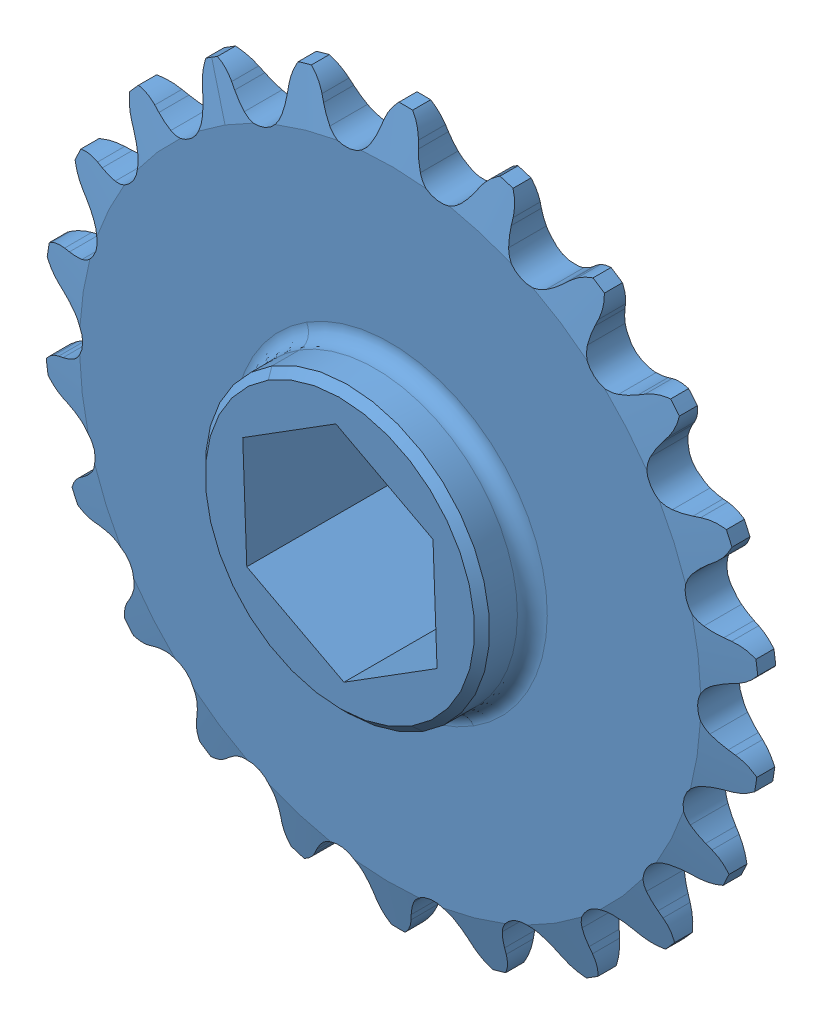
SolidWorks assembly WCP - GreyT Elevator (Cascade, 2 Stage) (1).step, configuration Default. Lengths in mm.
Overall size (65.87 65.96 9.52).
407 component instances, 66 part files, 0 mates.
Components (placement in the parent):
- WCP-0323 - Elevator Clamping Block.step-1: WCP-0323 - Elevator Clamping Block.step [Default] at (152.3365 1149.35 -25.4) x (0 0 1) z (-1 0 0) size (29.22 25.41 49.35) (hidden)
  - WCP-0323-001 Rev2.step-1: WCP-0323-001 Rev2.step [Default] at origin size (20.38 25.41 40.49)
  - WCP-0498 Rev1.step-1: WCP-0498 Rev1.step [Default] at (2.254 0 6.7) x (0 0.307359 0.951594) z (-1 0 0) size (12 12 4)
  - WCP-0212_0_250_radial_bearing.step-1: WCP-0212_0_250_radial_bearing.step [Default] at (-9.525 0 15.4781) size (19.05 19.05 7.14)
  - WCP-0473 Rev1.step-1: WCP-0473 Rev1.step [Default] at (-9.525 0 10.4394) x (-0.082744 -0.996571 0) z (-0.996571 0.082744 0) size (9.53 20.65 9.53)
  - #8-32 x .25L BHCS.step-1: #8-32 x .25L BHCS.step [Default] at (6.7178 0 6.7) x (0 -0.337236 -0.94142) z (1 0 0) size (10.28 8 12.02)
- WCP-0323 - Elevator Clamping Block-1.step-1: WCP-0323 - Elevator Clamping Block-1.step [Default] at (152.3365 1149.35 25.4) x (0 0 -1) z (-1 0 0) size (29.22 25.41 49.35) (hidden)
  - WCP-0323-001 Rev2.step-1: WCP-0323-001 Rev2.step [Default] at origin size (20.38 25.41 40.49)
  - WCP-0498 Rev1.step-1: WCP-0498 Rev1.step [Default] at (2.254 0 6.7) x (0 0.307359 0.951594) z (-1 0 0) size (12 12 4)
  - WCP-0212_0_250_radial_bearing.step-1: WCP-0212_0_250_radial_bearing.step [Default] at (-9.525 0 15.4781) size (19.05 19.05 7.14)
  - WCP-0473 Rev1.step-1: WCP-0473 Rev1.step [Default] at (-9.525 0 10.4394) x (-0.082744 -0.996571 0) z (-0.996571 0.082744 0) size (9.53 20.65 9.53)
  - #8-32 x .25L BHCS.step-1: #8-32 x .25L BHCS.step [Default] at (6.7178 0 6.7) x (0 -0.337236 -0.94142) z (1 0 0) size (10.28 8 12.02)
- WCP-0323 - Elevator Clamping Block-2.step-1: WCP-0323 - Elevator Clamping Block-2.step [Default] at (139.7635 57.15 25.4) x (0 0 -1) z (1 0 0) size (29.22 25.41 49.35) (hidden)
  - WCP-0323-001 Rev2.step-1: WCP-0323-001 Rev2.step [Default] at origin size (20.38 25.41 40.49)
  - WCP-0498 Rev1.step-1: WCP-0498 Rev1.step [Default] at (2.254 0 6.7) x (0 0.307359 0.951594) z (-1 0 0) size (12 12 4)
  - WCP-0212_0_250_radial_bearing.step-1: WCP-0212_0_250_radial_bearing.step [Default] at (-9.525 0 15.4781) size (19.05 19.05 7.14)
  - WCP-0473 Rev1.step-1: WCP-0473 Rev1.step [Default] at (-9.525 0 10.4394) x (-0.082744 -0.996571 0) z (-0.996571 0.082744 0) size (9.53 20.65 9.53)
  - #8-32 x .25L BHCS.step-1: #8-32 x .25L BHCS.step [Default] at (6.7178 0 6.7) x (0 -0.337236 -0.94142) z (1 0 0) size (10.28 8 12.02)
- WCP-0323 - Elevator Clamping Block-3.step-1: WCP-0323 - Elevator Clamping Block-3.step [Default] at (139.7635 57.15 -25.4) x (0 0 1) z (1 0 0) size (29.22 25.41 49.35) (hidden)
  - WCP-0323-001 Rev2.step-1: WCP-0323-001 Rev2.step [Default] at origin size (20.38 25.41 40.49)
  - WCP-0498 Rev1.step-1: WCP-0498 Rev1.step [Default] at (2.254 0 6.7) x (0 0.307359 0.951594) z (-1 0 0) size (12 12 4)
  - WCP-0212_0_250_radial_bearing.step-1: WCP-0212_0_250_radial_bearing.step [Default] at (-9.525 0 15.4781) size (19.05 19.05 7.14)
  - WCP-0473 Rev1.step-1: WCP-0473 Rev1.step [Default] at (-9.525 0 10.4394) x (-0.082744 -0.996571 0) z (-0.996571 0.082744 0) size (9.53 20.65 9.53)
  - #8-32 x .25L BHCS.step-1: #8-32 x .25L BHCS.step [Default] at (6.7178 0 6.7) x (0 -0.337236 -0.94142) z (1 0 0) size (10.28 8 12.02)
- WCP-0323 - Elevator Clamping Block-4.step-1: WCP-0323 - Elevator Clamping Block-4.step [Default] at (101.6635 82.55 25.4) x (0 0 -1) z (1 0 0) size (29.22 25.41 49.35) (hidden)
  - WCP-0323-001 Rev2.step-1: WCP-0323-001 Rev2.step [Default] at origin size (20.38 25.41 40.49)
  - WCP-0498 Rev1.step-1: WCP-0498 Rev1.step [Default] at (2.254 0 6.7) x (0 0.307359 0.951594) z (-1 0 0) size (12 12 4)
  - WCP-0212_0_250_radial_bearing.step-1: WCP-0212_0_250_radial_bearing.step [Default] at (-9.525 0 15.4781) size (19.05 19.05 7.14)
  - WCP-0473 Rev1.step-1: WCP-0473 Rev1.step [Default] at (-9.525 0 10.4394) x (-0.082744 -0.996571 0) z (-0.996571 0.082744 0) size (9.53 20.65 9.53)
  - #8-32 x .25L BHCS.step-1: #8-32 x .25L BHCS.step [Default] at (6.7178 0 6.7) x (0 -0.337236 -0.94142) z (1 0 0) size (10.28 8 12.02)
- WCP-0323 - Elevator Clamping Block-5.step-1: WCP-0323 - Elevator Clamping Block-5.step [Default] at (101.6635 82.55 -25.4) x (0 0 1) z (1 0 0) size (29.22 25.41 49.35) (hidden)
  - WCP-0323-001 Rev2.step-1: WCP-0323-001 Rev2.step [Default] at origin size (20.38 25.41 40.49)
  - WCP-0498 Rev1.step-1: WCP-0498 Rev1.step [Default] at (2.254 0 6.7) x (0 0.307359 0.951594) z (-1 0 0) size (12 12 4)
  - WCP-0212_0_250_radial_bearing.step-1: WCP-0212_0_250_radial_bearing.step [Default] at (-9.525 0 15.4781) size (19.05 19.05 7.14)
  - WCP-0473 Rev1.step-1: WCP-0473 Rev1.step [Default] at (-9.525 0 10.4394) x (-0.082744 -0.996571 0) z (-0.996571 0.082744 0) size (9.53 20.65 9.53)
  - #8-32 x .25L BHCS.step-1: #8-32 x .25L BHCS.step [Default] at (6.7178 0 6.7) x (0 -0.337236 -0.94142) z (1 0 0) size (10.28 8 12.02)
- WCP-0323 - Elevator Clamping Block-6.step-1: WCP-0323 - Elevator Clamping Block-6.step [Default] at (101.6635 222.25 25.4) x (0 0 -1) z (1 0 0) size (29.22 25.41 49.35) (hidden)
  - WCP-0323-001 Rev2.step-1: WCP-0323-001 Rev2.step [Default] at origin size (20.38 25.41 40.49)
  - WCP-0498 Rev1.step-1: WCP-0498 Rev1.step [Default] at (2.254 0 6.7) x (0 0.307359 0.951594) z (-1 0 0) size (12 12 4)
  - WCP-0212_0_250_radial_bearing.step-1: WCP-0212_0_250_radial_bearing.step [Default] at (-9.525 0 15.4781) size (19.05 19.05 7.14)
  - WCP-0473 Rev1.step-1: WCP-0473 Rev1.step [Default] at (-9.525 0 10.4394) x (-0.082744 -0.996571 0) z (-0.996571 0.082744 0) size (9.53 20.65 9.53)
  - #8-32 x .25L BHCS.step-1: #8-32 x .25L BHCS.step [Default] at (6.7178 0 6.7) x (0 -0.337236 -0.94142) z (1 0 0) size (10.28 8 12.02)
- WCP-0323 - Elevator Clamping Block-7.step-1: WCP-0323 - Elevator Clamping Block-7.step [Default] at (101.6635 222.25 -25.4) x (0 0 1) z (1 0 0) size (29.22 25.41 49.35) (hidden)
  - WCP-0323-001 Rev2.step-1: WCP-0323-001 Rev2.step [Default] at origin size (20.38 25.41 40.49)
  - WCP-0498 Rev1.step-1: WCP-0498 Rev1.step [Default] at (2.254 0 6.7) x (0 0.307359 0.951594) z (-1 0 0) size (12 12 4)
  - WCP-0212_0_250_radial_bearing.step-1: WCP-0212_0_250_radial_bearing.step [Default] at (-9.525 0 15.4781) size (19.05 19.05 7.14)
  - WCP-0473 Rev1.step-1: WCP-0473 Rev1.step [Default] at (-9.525 0 10.4394) x (-0.082744 -0.996571 0) z (-0.996571 0.082744 0) size (9.53 20.65 9.53)
  - #8-32 x .25L BHCS.step-1: #8-32 x .25L BHCS.step [Default] at (6.7178 0 6.7) x (0 -0.337236 -0.94142) z (1 0 0) size (10.28 8 12.02)
- WCP-0248 Rev1 - #35 Chain Turnbuckle.step-1: WCP-0248 Rev1 - #35 Chain Turnbuckle.step [Default] at (88.9 1124.7437 -66.675) x (0 -1 0) z (0 0 1) size (55.56 15.05 15.04) (hidden)
  - WCP-0247-001 Rev1.step-1: WCP-0247-001 Rev1.step [Default] at origin size (30.16 9.53 11)
  - NFS-0040_#10-32_jam_nut_left_hand_99961A520.step-1: NFS-0040_#10-32_jam_nut_left_hand_99961A520.step [Default] at (-16.6687 0 0) x (0 0.5 -0.866025) z (0 0.866025 0.5) size (11.01 3.2 11.02)
  - NFS-0037_#10-32_jam_nut_90480A195.step-1: NFS-0037_#10-32_jam_nut_90480A195.step [Default] at (16.6687 0 0) x (0 0.5 0.866025) z (0 -0.866025 0.5) size (11.01 3.2 11.02)
  - WCP-0248-001 Rev1.step-1: WCP-0248-001 Rev1.step [Default] at (23.8125 0 0) x (0 0 1) z (0 1 0) size (9 25.4 9)
  - WCP-0248-002 Rev1.step-1: WCP-0248-002 Rev1.step [Default] at (-23.8125 0 0) x (0 0 -1) z (0 1 0) size (9 25.4 9)
- WCP-0247 Rev1 - #25 Chain Turnbuckle.step-1: WCP-0247 Rev1 - #25 Chain Turnbuckle.step [Default] at (-47.6339 1117.6 -50.8) x (0 1 0) z (-1 0 0) size (50.8 15.05 15.04) (hidden)
  - WCP-0247-001 Rev1.step-1: WCP-0247-001 Rev1.step [Default] at origin size (30.16 9.53 11)
  - NFS-0040_#10-32_jam_nut_left_hand_99961A520.step-1: NFS-0040_#10-32_jam_nut_left_hand_99961A520.step [Default] at (-16.6687 0 0) x (0 0.5 -0.866025) z (0 0.866025 0.5) size (11.01 3.2 11.02)
  - NFS-0037_#10-32_jam_nut_90480A195.step-1: NFS-0037_#10-32_jam_nut_90480A195.step [Default] at (16.6687 0 0) x (0 0.5 0.866025) z (0 -0.866025 0.5) size (11.01 3.2 11.02)
  - WCP-0247-002 Rev2.step-1: WCP-0247-002 Rev2.step [Default] at (22.225 0 0) x (0 0 1) z (0 1 0) size (9 23.02 5.21)
  - WCP-0247-003 Rev2.step-1: WCP-0247-003 Rev2.step [Default] at (-22.225 0 0) x (0 0 -1) z (0 1 0) size (9 23.02 5.21)
- WCP-0323 - Elevator Clamping Block-8.step-1: WCP-0323 - Elevator Clamping Block-8.step [Default] at (-152.3365 1149.35 25.4) x (0 0 -1) z (1 0 0) size (29.22 25.41 49.35) (hidden)
  - WCP-0323-001 Rev2.step-1: WCP-0323-001 Rev2.step [Default] at origin size (20.38 25.41 40.49)
  - WCP-0498 Rev1.step-1: WCP-0498 Rev1.step [Default] at (2.254 0 6.7) x (0 0.307359 0.951594) z (-1 0 0) size (12 12 4)
  - WCP-0212_0_250_radial_bearing.step-1: WCP-0212_0_250_radial_bearing.step [Default] at (-9.525 0 15.4781) size (19.05 19.05 7.14)
  - WCP-0473 Rev1.step-1: WCP-0473 Rev1.step [Default] at (-9.525 0 10.4394) x (-0.082744 -0.996571 0) z (-0.996571 0.082744 0) size (9.53 20.65 9.53)
  - #8-32 x .25L BHCS.step-1: #8-32 x .25L BHCS.step [Default] at (6.7178 0 6.7) x (0 -0.337236 -0.94142) z (1 0 0) size (10.28 8 12.02)
- WCP-0323 - Elevator Clamping Block-9.step-1: WCP-0323 - Elevator Clamping Block-9.step [Default] at (-152.3365 1149.35 -25.4) x (0 0 1) z (1 0 0) size (29.22 25.41 49.35) (hidden)
  - WCP-0323-001 Rev2.step-1: WCP-0323-001 Rev2.step [Default] at origin size (20.38 25.41 40.49)
  - WCP-0498 Rev1.step-1: WCP-0498 Rev1.step [Default] at (2.254 0 6.7) x (0 0.307359 0.951594) z (-1 0 0) size (12 12 4)
  - WCP-0212_0_250_radial_bearing.step-1: WCP-0212_0_250_radial_bearing.step [Default] at (-9.525 0 15.4781) size (19.05 19.05 7.14)
  - WCP-0473 Rev1.step-1: WCP-0473 Rev1.step [Default] at (-9.525 0 10.4394) x (-0.082744 -0.996571 0) z (-0.996571 0.082744 0) size (9.53 20.65 9.53)
  - #8-32 x .25L BHCS.step-1: #8-32 x .25L BHCS.step [Default] at (6.7178 0 6.7) x (0 -0.337236 -0.94142) z (1 0 0) size (10.28 8 12.02)
- WCP-0583 Rev1 - Cascade Pulley Block.step-1: WCP-0583 Rev1 - Cascade Pulley Block.step [Default] at (88.9 25.4 -25.4) x (1 0 0) z (0 1 0) size (47.02 52.05 52.05) (hidden)
  - WCP-0096 Rev6.step-1: WCP-0096 Rev6.step [Default] at (0 25.4 6.35) size (12.65 52.05 52.05)
    - WCP-0096-001 Rev6.step-1: WCP-0096-001 Rev6.step [Default] at origin size (7.57 38.1 38.1)
    - WCP-0096-001 Rev6.step-2: WCP-0096-001 Rev6.step [Default] x (-1 0 0) z (0 0.866025 -0.5) size (7.57 38.1 38.1)
    - WCP-0356 Rev1.step-1: WCP-0356 Rev1.step [Default] at (0.4817 -4.7625 -8.2489) x (0 -0.126969 0.991907) z (0 -0.991907 -0.126969) size (4.06 11.05 4.06)
    - WCP-0356 Rev1.step-2: WCP-0356 Rev1.step [Default] at (0.4817 9.525 0) x (0 0.866766 0.498715) z (0 -0.498715 0.866766) size (4.06 11.05 4.06)
    - WCP-0356 Rev1.step-3: WCP-0356 Rev1.step [Default] at (0.4817 -4.7625 8.2489) x (0 -0.994015 -0.109248) z (0 0.109248 -0.994015) size (4.06 11.05 4.06)
    - WCP-0356 Rev1.step-4: WCP-0356 Rev1.step [Default] at (-0.4817 4.7625 -8.2489) x (0 -0.997555 0.069879) z (0 0.069879 0.997555) size (4.06 11.05 4.06)
    - WCP-0356 Rev1.step-5: WCP-0356 Rev1.step [Default] at (-0.4817 4.7625 8.2489) x (0 -0.7202 -0.693767) z (0 -0.693767 0.7202) size (4.06 11.05 4.06)
    - WCP-0356 Rev1.step-6: WCP-0356 Rev1.step [Default] at (-0.4817 -9.525 0) x (0 -0.997555 0.069879) z (0 0.069879 0.997555) size (4.06 11.05 4.06)
  - WCP-0583-001 Rev1.step-1: WCP-0583-001 Rev1.step [Default] at origin size (34.92 31.75 25.4)
  - WCP-0567 Rev1.step-1: WCP-0567 Rev1.step [Default] at (-6.3246 25.4 6.35) x (0 0 1) z (-1 0 0) size (15.88 15.88 7.94)
  - WCP-0567 Rev1.step-2: WCP-0567 Rev1.step [Default] at (6.3246 25.4 6.35) x (0 0 1) z (1 0 0) size (15.88 15.88 7.94)
  - WCP-0203 Rev1.step-1: WCP-0203 Rev1.step [Default] at (0 25.4 6.35) size (15.88 9.5 9.5)
  - 10-32 BHCS - No Thread_WCP-0258 - 1.750.step-1: 10-32 BHCS - No Thread_WCP-0258 - 1.750.step [Default] at (-17.4625 25.4 6.35) x (0 -0.816967 0.576685) z (0 -0.576685 -0.816967) size (9.17 47.02 9.17)
  - WCP-0326 Rev1.step-1: WCP-0326 Rev1.step [Default] at (19.8374 25.4 6.35) x (0 0.003214 -0.999995) z (0 -0.999995 -0.003214) size (11.02 4.76 11)
- WCP-0583 Rev1 - Cascade Pulley Block-1.step-1: WCP-0583 Rev1 - Cascade Pulley Block-1.step [Default] at (88.9 1219.2 -25.4) x (1 0 0) z (0 1 0) size (47.02 52.05 52.05) (hidden)
  - WCP-0096 Rev6-1.step-1: WCP-0096 Rev6-1.step [Default] at (0 25.4 6.35) size (12.65 52.05 52.05)
    - WCP-0096-001 Rev6.step-1: WCP-0096-001 Rev6.step [Default] at origin size (7.57 38.1 38.1)
    - WCP-0096-001 Rev6.step-2: WCP-0096-001 Rev6.step [Default] x (-1 0 0) z (0 0.866025 -0.5) size (7.57 38.1 38.1)
    - WCP-0356 Rev1.step-1: WCP-0356 Rev1.step [Default] at (0.4817 -4.7625 -8.2489) x (0 -0.126969 0.991907) z (0 -0.991907 -0.126969) size (4.06 11.05 4.06)
    - WCP-0356 Rev1.step-2: WCP-0356 Rev1.step [Default] at (0.4817 9.525 0) x (0 0.866766 0.498715) z (0 -0.498715 0.866766) size (4.06 11.05 4.06)
    - WCP-0356 Rev1.step-3: WCP-0356 Rev1.step [Default] at (0.4817 -4.7625 8.2489) x (0 -0.994015 -0.109248) z (0 0.109248 -0.994015) size (4.06 11.05 4.06)
    - WCP-0356 Rev1.step-4: WCP-0356 Rev1.step [Default] at (-0.4817 4.7625 -8.2489) x (0 -0.997555 0.069879) z (0 0.069879 0.997555) size (4.06 11.05 4.06)
    - WCP-0356 Rev1.step-5: WCP-0356 Rev1.step [Default] at (-0.4817 4.7625 8.2489) x (0 -0.7202 -0.693767) z (0 -0.693767 0.7202) size (4.06 11.05 4.06)
    - WCP-0356 Rev1.step-6: WCP-0356 Rev1.step [Default] at (-0.4817 -9.525 0) x (0 -0.997555 0.069879) z (0 0.069879 0.997555) size (4.06 11.05 4.06)
  - WCP-0583-001 Rev1.step-1: WCP-0583-001 Rev1.step [Default] at origin size (34.92 31.75 25.4)
  - WCP-0567 Rev1.step-1: WCP-0567 Rev1.step [Default] at (-6.3246 25.4 6.35) x (0 0 1) z (-1 0 0) size (15.88 15.88 7.94)
  - WCP-0567 Rev1.step-2: WCP-0567 Rev1.step [Default] at (6.3246 25.4 6.35) x (0 0 1) z (1 0 0) size (15.88 15.88 7.94)
  - WCP-0203 Rev1.step-1: WCP-0203 Rev1.step [Default] at (0 25.4 6.35) size (15.88 9.5 9.5)
  - 10-32 BHCS - No Thread_WCP-0258 - 1.750.step-1: 10-32 BHCS - No Thread_WCP-0258 - 1.750.step [Default] at (-17.4625 25.4 6.35) x (0 -0.816967 0.576685) z (0 -0.576685 -0.816967) size (9.17 47.02 9.17)
  - WCP-0326 Rev1.step-1: WCP-0326 Rev1.step [Default] at (19.8374 25.4 6.35) x (0 0.003214 -0.999995) z (0 -0.999995 -0.003214) size (11.02 4.76 11)
- WCP-0583 Rev1 - Cascade Pulley Block_Mirrored.step-1: WCP-0583 Rev1 - Cascade Pulley Block_Mirrored.step [Default] at (-88.9 1219.2 -25.4) x (1 0 0) z (0 1 0) size (47.02 52.05 52.05) (hidden)
  - WCP-0096 Rev6-2.step-1: WCP-0096 Rev6-2.step [Default] at (0 25.4 6.35) size (12.65 52.05 52.05)
    - WCP-0096-001 Rev6.step-1: WCP-0096-001 Rev6.step [Default] at origin size (7.57 38.1 38.1)
    - WCP-0096-001 Rev6.step-2: WCP-0096-001 Rev6.step [Default] x (-1 0 0) z (0 0.866025 -0.5) size (7.57 38.1 38.1)
    - WCP-0356 Rev1.step-1: WCP-0356 Rev1.step [Default] at (0.4817 -4.7625 -8.2489) x (0 -0.126969 0.991907) z (0 -0.991907 -0.126969) size (4.06 11.05 4.06)
    - WCP-0356 Rev1.step-2: WCP-0356 Rev1.step [Default] at (0.4817 9.525 0) x (0 0.866766 0.498715) z (0 -0.498715 0.866766) size (4.06 11.05 4.06)
    - WCP-0356 Rev1.step-3: WCP-0356 Rev1.step [Default] at (0.4817 -4.7625 8.2489) x (0 -0.994015 -0.109248) z (0 0.109248 -0.994015) size (4.06 11.05 4.06)
    - WCP-0356 Rev1.step-4: WCP-0356 Rev1.step [Default] at (-0.4817 4.7625 -8.2489) x (0 -0.997555 0.069879) z (0 0.069879 0.997555) size (4.06 11.05 4.06)
    - WCP-0356 Rev1.step-5: WCP-0356 Rev1.step [Default] at (-0.4817 4.7625 8.2489) x (0 -0.7202 -0.693767) z (0 -0.693767 0.7202) size (4.06 11.05 4.06)
    - WCP-0356 Rev1.step-6: WCP-0356 Rev1.step [Default] at (-0.4817 -9.525 0) x (0 -0.997555 0.069879) z (0 0.069879 0.997555) size (4.06 11.05 4.06)
  - WCP-0583-001 Rev1.step-1: WCP-0583-001 Rev1.step [Default] at origin size (34.92 31.75 25.4)
  - WCP-0567 Rev1.step-1: WCP-0567 Rev1.step [Default] at (-6.3246 25.4 6.35) x (0 0 1) z (-1 0 0) size (15.88 15.88 7.94)
  - WCP-0567 Rev1.step-2: WCP-0567 Rev1.step [Default] at (6.3246 25.4 6.35) x (0 0 1) z (1 0 0) size (15.88 15.88 7.94)
  - WCP-0203 Rev1.step-1: WCP-0203 Rev1.step [Default] at (0 25.4 6.35) size (15.88 9.5 9.5)
  - 10-32 BHCS - No Thread_WCP-0258 - 1.750.step-1: 10-32 BHCS - No Thread_WCP-0258 - 1.750.step [Default] at (17.4625 25.4 6.35) x (0 0.844944 -0.534854) z (0 -0.534854 -0.844944) size (9.17 47.02 9.17)
  - WCP-0326 Rev1.step-1: WCP-0326 Rev1.step [Default] at (-19.8374 25.4 6.35) x (0 -0.925447 -0.378877) z (0 0.378877 -0.925447) size (11.02 4.76 11)
- WCP-0583 Rev1 - Cascade Pulley Block_Mirrored-1.step-1: WCP-0583 Rev1 - Cascade Pulley Block_Mirrored-1.step [Default] at (-88.9 25.4 -25.4) x (1 0 0) z (0 1 0) size (47.02 52.05 52.05) (hidden)
  - WCP-0096 Rev6-3.step-1: WCP-0096 Rev6-3.step [Default] at (0 25.4 6.35) size (12.65 52.05 52.05)
    - WCP-0096-001 Rev6.step-1: WCP-0096-001 Rev6.step [Default] at origin size (7.57 38.1 38.1)
    - WCP-0096-001 Rev6.step-2: WCP-0096-001 Rev6.step [Default] x (-1 0 0) z (0 0.866025 -0.5) size (7.57 38.1 38.1)
    - WCP-0356 Rev1.step-1: WCP-0356 Rev1.step [Default] at (0.4817 -4.7625 -8.2489) x (0 -0.126969 0.991907) z (0 -0.991907 -0.126969) size (4.06 11.05 4.06)
    - WCP-0356 Rev1.step-2: WCP-0356 Rev1.step [Default] at (0.4817 9.525 0) x (0 0.866766 0.498715) z (0 -0.498715 0.866766) size (4.06 11.05 4.06)
    - WCP-0356 Rev1.step-3: WCP-0356 Rev1.step [Default] at (0.4817 -4.7625 8.2489) x (0 -0.994015 -0.109248) z (0 0.109248 -0.994015) size (4.06 11.05 4.06)
    - WCP-0356 Rev1.step-4: WCP-0356 Rev1.step [Default] at (-0.4817 4.7625 -8.2489) x (0 -0.997555 0.069879) z (0 0.069879 0.997555) size (4.06 11.05 4.06)
    - WCP-0356 Rev1.step-5: WCP-0356 Rev1.step [Default] at (-0.4817 4.7625 8.2489) x (0 -0.7202 -0.693767) z (0 -0.693767 0.7202) size (4.06 11.05 4.06)
    - WCP-0356 Rev1.step-6: WCP-0356 Rev1.step [Default] at (-0.4817 -9.525 0) x (0 -0.997555 0.069879) z (0 0.069879 0.997555) size (4.06 11.05 4.06)
  - WCP-0583-001 Rev1.step-1: WCP-0583-001 Rev1.step [Default] at origin size (34.92 31.75 25.4)
  - WCP-0567 Rev1.step-1: WCP-0567 Rev1.step [Default] at (-6.3246 25.4 6.35) x (0 0 1) z (-1 0 0) size (15.88 15.88 7.94)
  - WCP-0567 Rev1.step-2: WCP-0567 Rev1.step [Default] at (6.3246 25.4 6.35) x (0 0 1) z (1 0 0) size (15.88 15.88 7.94)
  - WCP-0203 Rev1.step-1: WCP-0203 Rev1.step [Default] at (0 25.4 6.35) size (15.88 9.5 9.5)
  - 10-32 BHCS - No Thread_WCP-0258 - 1.750.step-1: 10-32 BHCS - No Thread_WCP-0258 - 1.750.step [Default] at (17.4625 25.4 6.35) x (0 0.844944 -0.534854) z (0 -0.534854 -0.844944) size (9.17 47.02 9.17)
  - WCP-0326 Rev1.step-1: WCP-0326 Rev1.step [Default] at (-19.8374 25.4 6.35) x (0 -0.925447 -0.378877) z (0 0.378877 -0.925447) size (11.02 4.76 11)
- WCP-0323 - Elevator Clamping Block-10.step-1: WCP-0323 - Elevator Clamping Block-10.step [Default] at (-139.7635 57.15 -25.4) x (0 0 1) z (-1 0 0) size (29.22 25.41 49.35) (hidden)
  - WCP-0323-001 Rev2.step-1: WCP-0323-001 Rev2.step [Default] at origin size (20.38 25.41 40.49)
  - WCP-0498 Rev1.step-1: WCP-0498 Rev1.step [Default] at (2.254 0 6.7) x (0 0.307359 0.951594) z (-1 0 0) size (12 12 4)
  - WCP-0212_0_250_radial_bearing.step-1: WCP-0212_0_250_radial_bearing.step [Default] at (-9.525 0 15.4781) size (19.05 19.05 7.14)
  - WCP-0473 Rev1.step-1: WCP-0473 Rev1.step [Default] at (-9.525 0 10.4394) x (-0.082744 -0.996571 0) z (-0.996571 0.082744 0) size (9.53 20.65 9.53)
  - #8-32 x .25L BHCS.step-1: #8-32 x .25L BHCS.step [Default] at (6.7178 0 6.7) x (0 -0.337236 -0.94142) z (1 0 0) size (10.28 8 12.02)
- WCP-0557 Rev1 - WCP Single Stage Gearbox_0.5_ Hex.step-1: WCP-0557 Rev1 - WCP Single Stage Gearbox_0.5_ Hex.step [Default] at (-25.4 0 66.675) x (-1 0 0) z (0 0 -1) size (173.55 82.41 254.05) (hidden)
  - WCP-0557-001 Rev1.step-1: WCP-0557-001 Rev1.step [Default] at origin size (151.92 76.2 6.35)
  - WCP-0557-002 Rev1.step-1: WCP-0557-002 Rev1.step [Default] at (0 0 34.925) size (76.2 76.2 6.35)
  - 217-6515_Falcon_500_Default_As Machined_.step-1: 217-6515_Falcon_500_Default_As Machined_.step [Default] at (45.7962 0 -29.375) x (0.866025 0.5 0) z (0 0 1) size (60 60 115.81)
  - 217-6515_Falcon_500_Default_As Machined_.step-2: 217-6515_Falcon_500_Default_As Machined_.step [Default] at (-45.7962 0 -29.375) x (0.866025 0.5 0) z (0 0 1) size (60 60 115.81)
  - 217-6919_Falcon_12T.step-1: 217-6919_Falcon_12T.step [Default] at (45.7962 0 12.5775) x (0.990666 -0.136309 0) z (0 0 1) size (17.78 17.78 19.05)
  - 217-6919_Falcon_12T.step-2: 217-6919_Falcon_12T.step [Default] at (-45.7962 0 12.5775) x (0.990666 -0.136309 0) z (0 0 1) size (17.78 17.78 19.05)
  - WCP-0226 Rev1.step-1: WCP-0226 Rev1.step [Default] at (32.5438 -32.5438 17.4625) x (0 0 -1) z (0.876265 0.481829 0) size (28.57 9.5 9.5)
  - WCP-0226 Rev1.step-2: WCP-0226 Rev1.step [Default] at (32.5438 32.5438 17.4625) x (0 0 -1) z (-0.524135 0.851635 0) size (28.57 9.5 9.5)
  - WCP-0226 Rev1.step-3: WCP-0226 Rev1.step [Default] at (-32.5438 -32.5438 17.4625) x (0 0 -1) z (0.876265 0.481829 0) size (28.57 9.5 9.5)
  - WCP-0226 Rev1.step-4: WCP-0226 Rev1.step [Default] at (-32.5438 32.5438 17.4625) x (0 0 -1) z (0.876265 0.481829 0) size (28.57 9.5 9.5)
  - WCP-0557-004 Rev1.step-1: WCP-0557-004 Rev1.step [Default] at (0 0 0.7937) x (1 0 0) z (0 -1 0) size (45 7.94 45)
  - WCP-0781_0_500_flanged_bearing.step-1: WCP-0781_0_500_flanged_bearing.step [Default] at (0 0 -3.175) x (0.999832 0.018325 0) z (0.018325 -0.999832 0) size (31.12 7.94 31.12)
  - WCP-0557-004 Rev1.step-2: WCP-0557-004 Rev1.step [Default] at (0 0 34.1313) x (1 0 0) z (0 1 0) size (45 7.94 45)
  - WCP-0790_500L_500_hex.step-1: WCP-0790_500L_500_hex.step [Default] at (0 0 23.7617) x (0.953738 0.300639 0) z (0 0 1) size (19.5 19.5 12.7)
  - 10-32 BHCS - No Thread_WCP-0257 - 1.500.step-1: 10-32 BHCS - No Thread_WCP-0257 - 1.500.step [Default] at (32.5438 32.5438 0) x (0.63562 -0.772002 0) z (0.772002 0.63562 0) size (9.17 40.67 9.17)
  - 10-32 BHCS - No Thread_WCP-0257 - 1.500.step-2: 10-32 BHCS - No Thread_WCP-0257 - 1.500.step [Default] at (-32.5438 32.5438 0) x (0.63562 -0.772002 0) z (0.772002 0.63562 0) size (9.17 40.67 9.17)
  - 10-32 BHCS - No Thread_WCP-0257 - 1.500.step-3: 10-32 BHCS - No Thread_WCP-0257 - 1.500.step [Default] at (32.5438 -32.5438 0) x (0.63562 -0.772002 0) z (0.772002 0.63562 0) size (9.17 40.67 9.17)
  - 10-32 BHCS - No Thread_WCP-0257 - 1.500.step-4: 10-32 BHCS - No Thread_WCP-0257 - 1.500.step [Default] at (-32.5438 -32.5438 0) x (0.63562 -0.772002 0) z (0.772002 0.63562 0) size (9.17 40.67 9.17)
  - 10-32 BHCS - No Thread_WCP-0253 - 0.500.step-1: 10-32 BHCS - No Thread_WCP-0253 - 0.500.step [Default] at (45.7962 25.4 3.175) x (0.313732 -0.949511 0) z (-0.949511 -0.313732 0) size (9.17 15.27 9.17)
  - 10-32 BHCS - No Thread_WCP-0253 - 0.500.step-2: 10-32 BHCS - No Thread_WCP-0253 - 0.500.step [Default] at (45.7962 -25.4 3.175) x (0.270491 -0.962723 0) z (-0.962723 -0.270491 0) size (9.17 15.27 9.17)
  - 10-32 BHCS - No Thread_WCP-0253 - 0.500.step-3: 10-32 BHCS - No Thread_WCP-0253 - 0.500.step [Default] at (-45.7962 25.4 3.175) x (0.363225 -0.931702 0) z (-0.931702 -0.363225 0) size (9.17 15.27 9.17)
  - 10-32 BHCS - No Thread_WCP-0253 - 0.500.step-4: 10-32 BHCS - No Thread_WCP-0253 - 0.500.step [Default] at (-45.7962 -25.4 3.175) x (0.510832 -0.85968 0) z (-0.85968 -0.510832 0) size (9.17 15.27 9.17)
  - WCP-0832 Rev1.step-1: WCP-0832 Rev1.step [Default] at (0 0 87.3125) x (0.457904 0.889002 0) z (0 0 1) size (13.75 13.61 175.64)
  - WCP-0785_0_500_flanged_thunderhex_bearing.step-1: WCP-0785_0_500_flanged_thunderhex_bearing.step [Default] at (0 0 34.1313) x (-0.110978 -0.993823 0) z (0 0 -1) size (31.12 31.12 7.94)
  - WCP-0229 Rev1.step-1: WCP-0229 Rev1.step [Default] at (0 0 -3.6195) x (0 0 1) z (-0.791548 -0.611107 0) size (0.89 16.1 14.34)
  - WCP-0187 Rev1.step-1: WCP-0187 Rev1.step [Default] at (0 0 11.0871) x (0.99882 0.048566 0) z (0 0 1) size (78.68 78.68 12.65)
- WCP-0323 - Elevator Clamping Block-11.step-1: WCP-0323 - Elevator Clamping Block-11.step [Default] at (-101.6635 82.55 -25.4) x (0 0 1) z (-1 0 0) size (29.22 25.41 49.35) (hidden)
  - WCP-0323-001 Rev2.step-1: WCP-0323-001 Rev2.step [Default] at origin size (20.38 25.41 40.49)
  - WCP-0498 Rev1.step-1: WCP-0498 Rev1.step [Default] at (2.254 0 6.7) x (0 0.307359 0.951594) z (-1 0 0) size (12 12 4)
  - WCP-0212_0_250_radial_bearing.step-1: WCP-0212_0_250_radial_bearing.step [Default] at (-9.525 0 15.4781) size (19.05 19.05 7.14)
  - WCP-0473 Rev1.step-1: WCP-0473 Rev1.step [Default] at (-9.525 0 10.4394) x (-0.082744 -0.996571 0) z (-0.996571 0.082744 0) size (9.53 20.65 9.53)
  - #8-32 x .25L BHCS.step-1: #8-32 x .25L BHCS.step [Default] at (6.7178 0 6.7) x (0 -0.337236 -0.94142) z (1 0 0) size (10.28 8 12.02)
- WCP-0323 - Elevator Clamping Block-12.step-1: WCP-0323 - Elevator Clamping Block-12.step [Default] at (-101.6635 82.55 25.4) x (0 0 -1) z (-1 0 0) size (29.22 25.41 49.35) (hidden)
  - WCP-0323-001 Rev2.step-1: WCP-0323-001 Rev2.step [Default] at origin size (20.38 25.41 40.49)
  - WCP-0498 Rev1.step-1: WCP-0498 Rev1.step [Default] at (2.254 0 6.7) x (0 0.307359 0.951594) z (-1 0 0) size (12 12 4)
  - WCP-0212_0_250_radial_bearing.step-1: WCP-0212_0_250_radial_bearing.step [Default] at (-9.525 0 15.4781) size (19.05 19.05 7.14)
  - WCP-0473 Rev1.step-1: WCP-0473 Rev1.step [Default] at (-9.525 0 10.4394) x (-0.082744 -0.996571 0) z (-0.996571 0.082744 0) size (9.53 20.65 9.53)
  - #8-32 x .25L BHCS.step-1: #8-32 x .25L BHCS.step [Default] at (6.7178 0 6.7) x (0 -0.337236 -0.94142) z (1 0 0) size (10.28 8 12.02)
- WCP-0323 - Elevator Clamping Block-13.step-1: WCP-0323 - Elevator Clamping Block-13.step [Default] at (-139.7635 57.15 25.4) x (0 0 -1) z (-1 0 0) size (29.22 25.41 49.35) (hidden)
  - WCP-0323-001 Rev2.step-1: WCP-0323-001 Rev2.step [Default] at origin size (20.38 25.41 40.49)
  - WCP-0498 Rev1.step-1: WCP-0498 Rev1.step [Default] at (2.254 0 6.7) x (0 0.307359 0.951594) z (-1 0 0) size (12 12 4)
  - WCP-0212_0_250_radial_bearing.step-1: WCP-0212_0_250_radial_bearing.step [Default] at (-9.525 0 15.4781) size (19.05 19.05 7.14)
  - WCP-0473 Rev1.step-1: WCP-0473 Rev1.step [Default] at (-9.525 0 10.4394) x (-0.082744 -0.996571 0) z (-0.996571 0.082744 0) size (9.53 20.65 9.53)
  - #8-32 x .25L BHCS.step-1: #8-32 x .25L BHCS.step [Default] at (6.7178 0 6.7) x (0 -0.337236 -0.94142) z (1 0 0) size (10.28 8 12.02)
- WCP-0323 - Elevator Clamping Block-14.step-1: WCP-0323 - Elevator Clamping Block-14.step [Default] at (-101.6635 222.25 -25.4) x (0 0 1) z (-1 0 0) size (29.22 25.41 49.35) (hidden)
  - WCP-0323-001 Rev2.step-1: WCP-0323-001 Rev2.step [Default] at origin size (20.38 25.41 40.49)
  - WCP-0498 Rev1.step-1: WCP-0498 Rev1.step [Default] at (2.254 0 6.7) x (0 0.307359 0.951594) z (-1 0 0) size (12 12 4)
  - WCP-0212_0_250_radial_bearing.step-1: WCP-0212_0_250_radial_bearing.step [Default] at (-9.525 0 15.4781) size (19.05 19.05 7.14)
  - WCP-0473 Rev1.step-1: WCP-0473 Rev1.step [Default] at (-9.525 0 10.4394) x (-0.082744 -0.996571 0) z (-0.996571 0.082744 0) size (9.53 20.65 9.53)
  - #8-32 x .25L BHCS.step-1: #8-32 x .25L BHCS.step [Default] at (6.7178 0 6.7) x (0 -0.337236 -0.94142) z (1 0 0) size (10.28 8 12.02)
- WCP-0323 - Elevator Clamping Block-15.step-1: WCP-0323 - Elevator Clamping Block-15.step [Default] at (-101.6635 222.25 25.4) x (0 0 -1) z (-1 0 0) size (29.22 25.41 49.35) (hidden)
  - WCP-0323-001 Rev2.step-1: WCP-0323-001 Rev2.step [Default] at origin size (20.38 25.41 40.49)
  - WCP-0498 Rev1.step-1: WCP-0498 Rev1.step [Default] at (2.254 0 6.7) x (0 0.307359 0.951594) z (-1 0 0) size (12 12 4)
  - WCP-0212_0_250_radial_bearing.step-1: WCP-0212_0_250_radial_bearing.step [Default] at (-9.525 0 15.4781) size (19.05 19.05 7.14)
  - WCP-0473 Rev1.step-1: WCP-0473 Rev1.step [Default] at (-9.525 0 10.4394) x (-0.082744 -0.996571 0) z (-0.996571 0.082744 0) size (9.53 20.65 9.53)
  - #8-32 x .25L BHCS.step-1: #8-32 x .25L BHCS.step [Default] at (6.7178 0 6.7) x (0 -0.337236 -0.94142) z (1 0 0) size (10.28 8 12.02)
- WCP-0248 Rev1 - #35 Chain Turnbuckle-1.step-1: WCP-0248 Rev1 - #35 Chain Turnbuckle-1.step [Default] at (-88.9 1124.7437 -66.675) x (0 -1 0) z (0 0 -1) size (55.56 15.05 15.04) (hidden)
  - WCP-0247-001 Rev1.step-1: WCP-0247-001 Rev1.step [Default] at origin size (30.16 9.53 11)
  - NFS-0040_#10-32_jam_nut_left_hand_99961A520.step-1: NFS-0040_#10-32_jam_nut_left_hand_99961A520.step [Default] at (-16.6687 0 0) x (0 0.5 -0.866025) z (0 0.866025 0.5) size (11.01 3.2 11.02)
  - NFS-0037_#10-32_jam_nut_90480A195.step-1: NFS-0037_#10-32_jam_nut_90480A195.step [Default] at (16.6687 0 0) x (0 0.5 0.866025) z (0 -0.866025 0.5) size (11.01 3.2 11.02)
  - WCP-0248-001 Rev1.step-1: WCP-0248-001 Rev1.step [Default] at (23.8125 0 0) x (0 0 1) z (0 1 0) size (9 25.4 9)
  - WCP-0248-002 Rev1.step-1: WCP-0248-002 Rev1.step [Default] at (-23.8125 0 0) x (0 0 -1) z (0 1 0) size (9 25.4 9)
- WCP-EX-0019-001.step-1: WCP-EX-0019-001.step [Default] x (1 0 0) z (0 -1 0) size (457.2 50.8 25.4) (hidden)
- WCP-EX-0019-003.step-1: WCP-EX-0019-003.step [Default] at (165.1 609.6 0) x (0 -1 0) z (1 0 0) size (1193.8 50.8 25.4) (hidden)
- WCP-EX-0019-002.step-1: WCP-EX-0019-002.step [Default] at (0 1181.1 -88.9) size (355.6 50.8 25.4) (hidden)
- WCP-EX-0019-004.step-1: WCP-EX-0019-004.step [Default] at (127 622.3 0) x (0 -1 0) z (-1 0 0) size (1219.2 50.8 25.4) (hidden)
- WCP-EX-0019-007.step-1: WCP-EX-0019-007.step [Default] at (0 25.4 0) x (1 0 0) z (0 -1 0) size (228.6 50.8 25.4) (hidden)
- WCP-EX-0019-007.step-2: WCP-EX-0019-007.step [Default] at (0 1219.2 0) x (1 0 0) z (0 -1 0) size (228.6 50.8 25.4) (hidden)
- WCP-EX-0019-005.step-1: WCP-EX-0019-005.step [Default] at (88.9 152.4 0) x (0 -1 0) z (-1 0 0) size (228.6 50.8 25.4) (hidden)
- WCP-EX-0019-006.step-1: WCP-EX-0019-006.step [Default] at (0 50.8 0) x (1 0 0) z (0 -1 0) size (152.4 50.8 25.4) (hidden)
- WCP-EX-0019-006.step-2: WCP-EX-0019-006.step [Default] at (0 254 0) x (1 0 0) z (0 -1 0) size (152.4 50.8 25.4) (hidden)
- WCP-EX-0019-003.step-2: WCP-EX-0019-003.step [Default] at (-165.1 609.6 0) x (0 -1 0) z (1 0 0) size (1193.8 50.8 25.4) (hidden)
- 10-32 BHCS - No Thread_WCP-0261 - 2.500.step-1: 10-32 BHCS - No Thread_WCP-0261 - 2.500.step [Default] at (165.1 1143 30.1625) x (0.999937 0.011255 0) z (0.011255 -0.999937 0) size (9.17 66.07 9.17) (hidden)
- 10-32 BHCS - No Thread_WCP-0261 - 2.500.step-2: 10-32 BHCS - No Thread_WCP-0261 - 2.500.step [Default] at (165.1 1155.7 -30.1625) x (-0.802481 0.596678 0) z (-0.596678 -0.802481 0) size (9.17 66.07 9.17) (hidden)
- 10-32 BHCS - No Thread_WCP-0261 - 2.500.step-3: 10-32 BHCS - No Thread_WCP-0261 - 2.500.step [Default] at (127 50.8 -30.1625) x (-0.742242 0.670132 0) z (-0.670132 -0.742242 0) size (9.17 66.07 9.17) (hidden)
- 10-32 BHCS - No Thread_WCP-0261 - 2.500.step-4: 10-32 BHCS - No Thread_WCP-0261 - 2.500.step [Default] at (127 63.5 30.1625) x (0.985295 -0.170861 0) z (-0.170861 -0.985295 0) size (9.17 66.07 9.17) (hidden)
- 10-32 BHCS - No Thread_WCP-0261 - 2.500.step-5: 10-32 BHCS - No Thread_WCP-0261 - 2.500.step [Default] at (88.9 76.2 -30.1625) x (-0.742242 0.670132 0) z (-0.670132 -0.742242 0) size (9.17 66.07 9.17) (hidden)
- 10-32 BHCS - No Thread_WCP-0261 - 2.500.step-6: 10-32 BHCS - No Thread_WCP-0261 - 2.500.step [Default] at (88.9 88.9 30.1625) x (0.985295 -0.170861 0) z (-0.170861 -0.985295 0) size (9.17 66.07 9.17) (hidden)
- 10-32 BHCS - No Thread_WCP-0261 - 2.500.step-7: 10-32 BHCS - No Thread_WCP-0261 - 2.500.step [Default] at (88.9 215.9 -30.1625) x (-0.742242 0.670132 0) z (-0.670132 -0.742242 0) size (9.17 66.07 9.17) (hidden)
- 10-32 BHCS - No Thread_WCP-0261 - 2.500.step-8: 10-32 BHCS - No Thread_WCP-0261 - 2.500.step [Default] at (88.9 228.6 30.1625) x (0.985295 -0.170861 0) z (-0.170861 -0.985295 0) size (9.17 66.07 9.17) (hidden)
- 10-32 SHCS - No Thread_WCP-0274 - 4.500.step-1: 10-32 SHCS - No Thread_WCP-0274 - 4.500.step [Default] at (165.1 1168.4 -77.7875) x (0.495006 -0.86889 0) z (0.86889 0.495006 0) size (7.67 119.13 7.67) (hidden)
- 10-32 SHCS - No Thread_WCP-0274 - 4.500.step-2: 10-32 SHCS - No Thread_WCP-0274 - 4.500.step [Default] at (165.1 1193.8 -77.7875) x (0.495006 -0.86889 0) z (0.86889 0.495006 0) size (7.67 119.13 7.67) (hidden)
